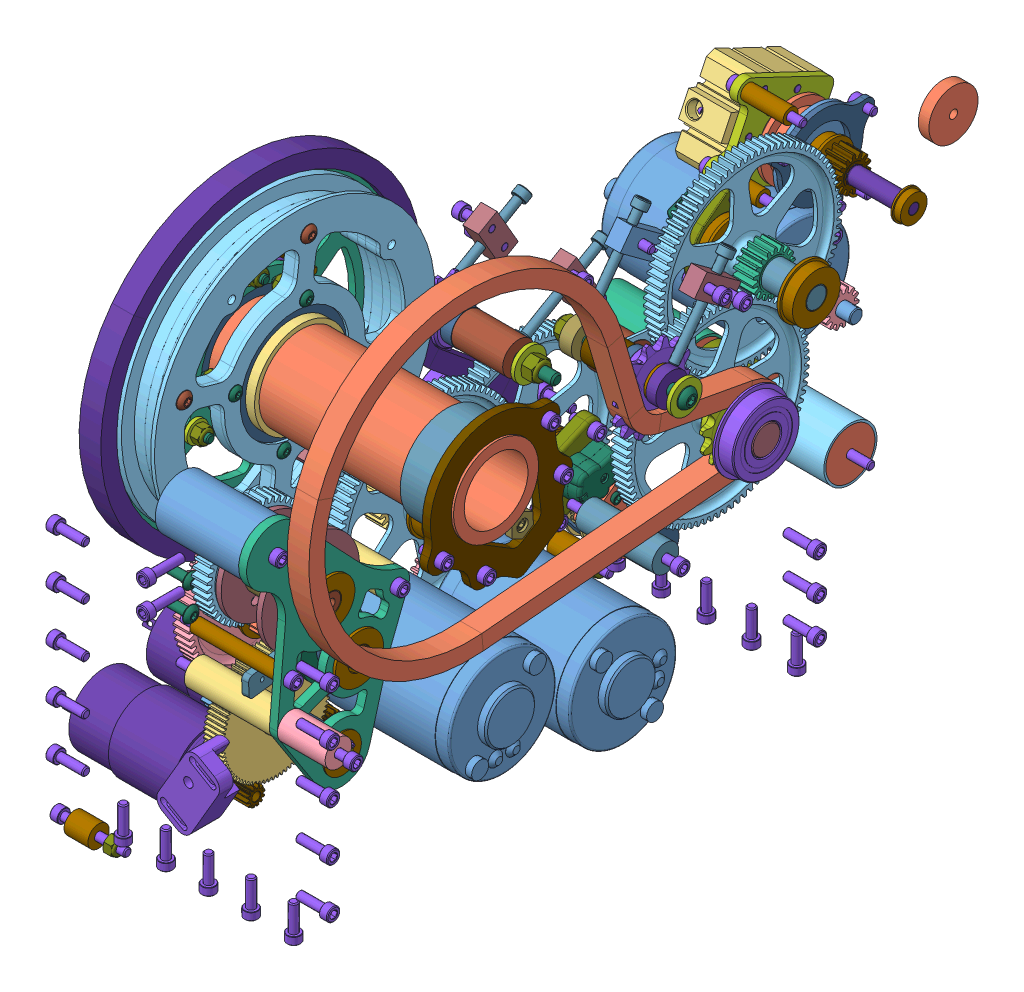
SolidWorks assembly 971-18-A-2900_Arm Gearbox, configuration Default. Lengths in mm. (continued)
Components (placement in the parent): (continued)
- SHCS-20: SHCS [0.4375, #10-32] at (157.9562 -11.0066 -39.4138) x (-1 0 0) z (0 -0.010983 -0.99994) size (16.17 7.92 7.92)
- SHCS-21: SHCS [0.4375, #10-32] at (157.9562 -40.3824 6.6222) x (-1 0 0) z (0 -0.010983 -0.99994) size (16.17 7.92 7.92)
- SHCS-22: SHCS [0.4375, #10-32] at (157.9562 -20.3652 31.9152) x (-1 0 0) z (0 -0.010983 -0.99994) size (16.17 7.92 7.92)
- SHCS-23: SHCS [0.4375, #10-32] at (0.7937 -20.3652 31.9152) x (1 0 0) z (0 -0.408057 0.912956) size (16.17 7.92 7.92)
- SHCS-24: SHCS [0.4375, #10-32] at (0.7937 -11.0066 -39.4138) x (1 0 0) z (0 -0.408057 0.912956) size (16.17 7.92 7.92)
- SHCS-25: SHCS [0.4375, #10-32] at (0.7937 -40.3824 6.6222) x (1 0 0) z (0 -0.408057 0.912956) size (16.17 7.92 7.92)
- SHCS-26: SHCS [0.4375, #10-32] at (0.7937 20.3652 -31.9152) x (1 0 0) z (0 -0.408057 0.912956) size (16.17 7.92 7.92)
- SHCS-27: SHCS [0.625, #10-32] at (150.8125 -172.339 95.6183) x (-1 0 0) z (0 -0.459114 -0.888377) size (20.93 7.92 7.92)
- SHCS-28: SHCS [0.625, #10-32] at (7.9375 -172.339 95.6183) x (1 0 0) z (0 0.669781 0.742559) size (20.93 7.92 7.92)
- SHCS-29: SHCS [0.625, #10-32] at (150.8125 -142.6527 95.6183) x (-1 0 0) z (0 -0.459114 -0.888377) size (20.93 7.92 7.92)
- SHCS-30: SHCS [0.625, #10-32] at (150.8125 -112.9665 95.6183) x (-1 0 0) z (0 -0.459114 -0.888377) size (20.93 7.92 7.92)
- SHCS-31: SHCS [0.625, #10-32] at (150.8125 -83.2802 95.6183) x (-1 0 0) z (0 -0.459114 -0.888377) size (20.93 7.92 7.92)
- SHCS-32: SHCS [0.625, #10-32] at (150.8125 -53.594 95.6183) x (-1 0 0) z (0 -0.459114 -0.888377) size (20.93 7.92 7.92)
- SHCS-33: SHCS [0.625, #10-32] at (7.9375 -142.6527 95.6183) x (1 0 0) z (0 0.669781 0.742559) size (20.93 7.92 7.92)
- SHCS-34: SHCS [0.625, #10-32] at (7.9375 -112.9665 95.6183) x (1 0 0) z (0 0.669781 0.742559) size (20.93 7.92 7.92)
- SHCS-35: SHCS [0.625, #10-32] at (7.9375 -83.2802 95.6183) x (1 0 0) z (0 0.669781 0.742559) size (20.93 7.92 7.92)
- SHCS-36: SHCS [0.625, #10-32] at (7.9375 -53.594 95.6183) x (1 0 0) z (0 0.669781 0.742559) size (20.93 7.92 7.92)
- SHCS-37: SHCS [0.625, #10-32] at (150.8125 -175.26 -195.2625) x (-1 0 0) z (0 -0.430535 -0.902574) size (20.93 7.92 7.92)
- SHCS-38: SHCS [0.625, #10-32] at (7.9375 -175.26 -195.2625) x (1 0 0) z (0 0.669781 0.742559) size (20.93 7.92 7.92)
- SHCS-39: SHCS [0.625, #10-32] at (7.9375 -152.7175 -195.2625) x (1 0 0) z (0 0.669781 0.742559) size (20.93 7.92 7.92)
- SHCS-40: SHCS [0.625, #10-32] at (7.9375 -130.175 -195.2625) x (1 0 0) z (0 0.669781 0.742559) size (20.93 7.92 7.92)
- SHCS-41: SHCS [0.625, #10-32] at (150.8125 -152.7175 -195.2625) x (-1 0 0) z (0 -0.430535 -0.902574) size (20.93 7.92 7.92)
- SHCS-42: SHCS [0.625, #10-32] at (150.8125 -130.175 -195.2625) x (-1 0 0) z (0 -0.430535 -0.902574) size (20.93 7.92 7.92)
- SHCS-46: SHCS [0.625, #10-32] at (139.6577 -185.0517 95.6183) x (0 1 0) z (-0.080041 0 -0.996792) size (20.93 7.92 7.92)
- SHCS-47: SHCS [0.625, #10-32] at (114.2153 -185.0517 95.6183) x (0 1 0) z (-0.080041 0 -0.996792) size (20.93 7.92 7.92)
- SHCS-48: SHCS [0.625, #10-32] at (88.773 -185.0517 95.6183) x (0 1 0) z (-0.266457 0 -0.963847) size (20.93 7.92 7.92)
- SHCS-49: SHCS [0.625, #10-32] at (63.3307 -185.0517 95.6183) x (0 1 0) z (-0.467971 0 -0.883744) size (20.93 7.92 7.92)
- SHCS-50: SHCS [0.625, #10-32] at (37.8883 -185.0517 95.6183) x (0 1 0) z (-0.662108 0 -0.749409) size (20.93 7.92 7.92)
- SHCS-52: SHCS [0.625, #10-32] at (122.2375 -186.4995 -195.2625) x (0 1 0) z (-0.080041 0 -0.996792) size (20.93 7.92 7.92)
- SHCS-53: SHCS [0.625, #10-32] at (95.25 -186.4995 -195.2625) x (0 1 0) z (-0.080041 0 -0.996792) size (20.93 7.92 7.92)
- SHCS-54: SHCS [0.625, #10-32] at (149.225 -186.4995 -195.2625) x (0 1 0) z (-0.266457 0 -0.963847) size (20.93 7.92 7.92)
- SHCS-55: SHCS [0.625, #10-32] at (68.2625 -186.4995 -195.2625) x (0 1 0) z (-0.467971 0 -0.883744) size (20.93 7.92 7.92)
- SHCS-56: SHCS [0.625, #10-32] at (41.275 -186.4995 -195.2625) x (0 1 0) z (-0.662108 0 -0.749409) size (20.93 7.92 7.92)
- SHCS-61: SHCS [1.5, #10-32] at (19.05 -204.4065 -195.2752) x (1 0 0) z (0 0.916141 -0.400857) size (43.15 7.92 7.92)
- No 10 Aluminum Spacer-8: No 10 Aluminum Spacer [0.5" OD, 0.5625" Length] at (13.4938 -204.4065 -195.2752) x (0 0.977573 -0.210597) z (1 0 0) size (12.7 12.7 14.29)
- SHCS-65: SHCS [0.625, #10-32] at (7.9375 -12.5246 -146.6125) x (1 0 0) z (0 -0.814974 -0.579498) size (20.93 7.92 7.92)
- SHCS-67: SHCS [0.625, #10-32] at (7.9375 -25.7229 -154.2325) x (1 0 0) z (0 -0.96514 -0.261734) size (20.93 7.92 7.92)
- SHCS-69: SHCS [0.625, #10-32] at (100.3427 21.0025 -150.0962) x (1 0 0) z (0 -0.52095 -0.853587) size (20.93 7.92 7.92)
- SHCS-71: SHCS [0.625, #10-32] at (100.3427 13.4742 -160.3243) x (1 0 0) z (0 -0.512621 -0.858615) size (20.93 7.92 7.92)
- 971-18-P-0243_Arm Gearbox Potentiometer Mount-2: 971-18-P-0243_Arm Gearbox Potentiometer Mount [Default] at (100.4062 -85.7984 -149.5368) x (0 0.994332 -0.106322) z (-1 0 0) size (42.8 25.4 21.27)
- VexPro_Hex Spacers-1: VexPro_Hex Spacers [1_2 Hex, 0.5] at (114.7839 -58.42 -165.2367) x (0 0 -1) z (1 0 0) size (19.51 19.51 12.7)
- SHCS-76: SHCS [0.625, #10-32] at (150.8125 29.2837 -138.8453) x (-1 0 0) z (0 -0.37606 -0.926595) size (20.93 7.92 7.92)
- SHCS-78: SHCS [0.625, #10-32] at (150.8125 20.2497 -151.119) x (-1 0 0) z (0 -0.490985 -0.871168) size (20.93 7.92 7.92)
- SHCS-80: SHCS [0.625, #10-32] at (60.325 -12.5246 -146.6125) x (-1 0 0) z (0 -0.909347 -0.416039) size (20.93 7.92 7.92)
- SHCS-82: SHCS [0.625, #10-32] at (60.325 -25.7229 -154.2325) x (-1 0 0) z (0 -0.967776 -0.251812) size (20.93 7.92 7.92)
- VexPro_Hex Spacers-2: VexPro_Hex Spacers [1_2 Hex, 0.0625] at (61.1187 -103.4997 -135.089) x (0 0.01328 -0.999912) z (1 0 0) size (19.51 19.51 1.59)
- 971-18-P-0249_Distal Shaft Spacer-1: 971-18-P-0249_Distal Shaft Spacer [Default] at (26.5543 -103.4997 -135.089) size (9.91 19.5 19.5)
- Nylon-Insert Locknut-3: Nylon-Insert Locknut [#8-32  Nylon-Insert Locknut] at (27.686 -204.4065 -195.2752) x (0 0.839079 -0.544009) z (0 -0.544009 -0.839079) size (8.73 5.95 10.08)
- No 10 Aluminum Spacer-9: No 10 Aluminum Spacer [0.5" OD, 0.5625" Length] at (13.4938 -204.4065 93.1418) x (0 0.977573 -0.210597) z (1 0 0) size (12.7 12.7 14.29)
- No 10 Aluminum Spacer-10: No 10 Aluminum Spacer [0.5" OD, 0.5625" Length] at (13.4938 -204.4065 -145.3959) x (0 0.977573 -0.210597) z (1 0 0) size (12.7 12.7 14.29)
- No 10 Aluminum Spacer-11: No 10 Aluminum Spacer [0.5" OD, 0.5625" Length] at (13.4938 -204.4065 -95.5167) x (0 0.977573 -0.210597) z (1 0 0) size (12.7 12.7 14.29)
- No 10 Aluminum Spacer-12: No 10 Aluminum Spacer [0.5" OD, 0.5625" Length] at (13.4938 -204.4065 -6.6167) x (0 0.977573 -0.210597) z (1 0 0) size (12.7 12.7 14.29)
- SHCS-84: SHCS [1.5, #10-32] at (19.05 -204.4065 93.1418) x (1 0 0) z (0 0.916141 -0.400857) size (43.15 7.92 7.92)
- SHCS-85: SHCS [1.5, #10-32] at (19.05 -204.4065 -145.3959) x (1 0 0) z (0 0.916141 -0.400857) size (43.15 7.92 7.92)
- SHCS-86: SHCS [1.5, #10-32] at (19.05 -204.4065 -95.5167) x (1 0 0) z (0 0.916141 -0.400857) size (43.15 7.92 7.92)
- SHCS-87: SHCS [1.5, #10-32] at (19.05 -204.4065 -6.6167) x (1 0 0) z (0 0.916141 -0.400857) size (43.15 7.92 7.92)
- Nylon-Insert Locknut-4: Nylon-Insert Locknut [#8-32  Nylon-Insert Locknut] at (27.686 -204.4065 93.1418) x (0 0.839079 -0.544009) z (0 -0.544009 -0.839079) size (8.73 5.95 10.08)
- Nylon-Insert Locknut-5: Nylon-Insert Locknut [#8-32  Nylon-Insert Locknut] at (27.686 -204.4065 -145.3959) x (0 0.839079 -0.544009) z (0 -0.544009 -0.839079) size (8.73 5.95 10.08)
- Nylon-Insert Locknut-6: Nylon-Insert Locknut [#8-32  Nylon-Insert Locknut] at (27.686 -204.4065 -95.5167) x (0 0.839079 -0.544009) z (0 -0.544009 -0.839079) size (8.73 5.95 10.08)
- Nylon-Insert Locknut-7: Nylon-Insert Locknut [#8-32  Nylon-Insert Locknut] at (27.686 -204.4065 -6.6167) x (0 0.839079 -0.544009) z (0 -0.544009 -0.839079) size (8.73 5.95 10.08)
- BHCS-3: BHCS [0.5625, #10-32] at (70.8279 -51.689 86.0933) x (0 -0.746359 0.665543) z (1 0 0) size (9.17 9.17 17.04)
- BHCS-4: BHCS [0.5625, #10-32] at (70.8279 -69.1515 86.0933) x (0 -0.746359 0.665543) z (1 0 0) size (9.17 9.17 17.04)
- SHCS-88: SHCS [0.75, #10-32] at (58.7375 -46.9265 90.8558) x (0 0 -1) z (0.742559 0.669781 0) size (24.1 7.92 7.92)
- SHCS-89: SHCS [0.75, #10-32] at (58.7375 -64.389 90.8558) x (0 0 -1) z (0.742559 0.669781 0) size (24.1 7.92 7.92)
- BHCS-6: BHCS [0.5, #10-32] at (77.2604 -134.8658 -152.2116) x (0 0.490356 0.871522) z (1 0 0) size (9.17 9.17 15.45)
- BHCS-7: BHCS [0.5, #10-32] at (77.2604 -128.7793 -160.3468) x (0 0.345971 0.938245) z (1 0 0) size (9.17 9.17 15.45)
- 91525A416_1-4 Oversized Washer-1: 91525A416_1-4 Oversized Washer [91525A416] at (-2.286 -39.637 -114.8895) size (2.29 19.05 19.05)
- 91525A416_1-4 Oversized Washer-2: 91525A416_1-4 Oversized Washer [91525A416] at (68.2625 -39.637 -114.8895) size (2.29 19.05 19.05)
- 91525A416_1-4 Oversized Washer-3: 91525A416_1-4 Oversized Washer [91525A416] at (158.75 -12.6592 -117.4327) size (2.29 19.05 19.05)
- 971-18-P-0057_Arm Gearbox Plates-2: 971-18-P-0057_Arm Gearbox Plates [Sponsor Pannel Outside] at (4.826 0 0) size (0.81 228.95 407.67) (hidden)
- 971-18-P-0057_Arm Gearbox Plates-3: 971-18-P-0057_Arm Gearbox Plates [Sponsor Pannel Inside] at (-4.826 0 0) size (0.81 222.6 407.67) (hidden)
- 971-18-P-0352_Arm Gearbox-Bumper Spacer-1: 971-18-P-0352_Arm Gearbox-Bumper Spacer [Default] at (90.8758 -115.2621 108.5723) x (0 0 -1) z (-0.864092 0.503334 0) size (17.72 44.45 22.86)
Mates (geometry in assembly coordinates):
- Concentric17: concentric anti-aligned: cylinder of MiniCIM-1 through (184.5808 -45.1539 -242.57) axis (-1 0 0) radius 32.131; cylinder of 971-18-P-0057_Arm Gearbox Plates-1 through (101.9302 -45.1539 -242.57) axis (1 0 0) radius 9.5631
- Concentric10: concentric anti-aligned: cylinder of MiniCIM-2 through (68.2625 -128.7803 -15.3525) axis (1 0 0) radius 4; cylinder of 14T-CIM_217-3414-1 through (44.9112 -128.7803 -15.3525) axis (-1 0 0) radius 4
- Concentric11: concentric anti-aligned: cylinder of 971-18-P-0057_Arm Gearbox Plates-1 through (68.2625 -91.1077 -64.9795) axis (-1 0 0) radius 14.2684; cylinder of 971-18-P-0186_84T Gear With Access Hole-2 through (49.2633 -91.1077 -64.9795) axis (1 0 0) radius 8.89
- Concentric21: concentric anti-aligned: cylinder of 971-18-P-0057_Arm Gearbox Plates-1 through (158.75 -58.42 -165.2367) axis (-1 0 0) radius 19.981; cylinder of 971-18-P-0186_84T Gear With Access Hole-4 through (121.1339 -58.42 -165.2367) axis (1 0 0) radius 8.89
- Concentric22: concentric anti-aligned: cylinder of 971-18-P-0057_Arm Gearbox Plates-1 through (158.75 -2.1568 -197.4778) axis (-1 0 0) radius 14.2684; cylinder of 18T-1_2-Hex-Steel_217-5460-2 through (121.1339 -2.1568 -197.4778) axis (1 0 0) radius 8.89
- Concentric12: concentric anti-aligned: cylinder of 28T-1_2-Hex-Steel_217-5468-1 through (49.2633 -91.1077 -64.9795) axis (-1 0 0) radius 8.89; cylinder of 971-18-P-0186_84T Gear With Access Hole-2 through (49.2633 -91.1077 -64.9795) axis (1 0 0) radius 8.89
- Concentric23: concentric aligned: cylinder of 971-18-P-0186_84T Gear With Access Hole-3 through (108.4848 -2.1568 -197.4778) axis (1 0 0) radius 8.89; cylinder of 18T-1_2-Hex-Steel_217-5460-2 through (121.1339 -2.1568 -197.4778) axis (1 0 0) radius 8.89
- Coincident29: coincident aligned: plane of 971-18-P-0186_84T Gear With Access Hole-4 through (121.1339 -58.42 -165.2367) normal (-1 0 0); plane of 18T-1_2-Hex-Steel_217-5460-2 through (121.1339 -2.1568 -197.4778) normal (-1 0 0)
- Coincident31: coordinate: point of 971-18-P-0057_Arm Gearbox Plates-1
- Concentric24: concentric anti-aligned: cylinder of 971-18-P-0057_Arm Gearbox Plates-1 through (6.35 0 0) axis (-1 0 0) radius 25; cylinder of 971-18-P-0063_Proximal Joint Chain-1 through (142.3112 0 0) axis (1 0 0) radius 95.7195
- Concentric30: concentric anti-aligned: cylinder of MiniCIM-3 through (68.2625 -149.225 -87.4394) axis (1 0 0) radius 4; cylinder of 14T-CIM_217-3414-2 through (44.9112 -149.225 -87.4394) axis (-1 0 0) radius 4
- Concentric31: concentric aligned: cylinder of MiniCIM-1 through (101.9302 -45.1539 -242.57) axis (-1 0 0) radius 4; cylinder of 14T-CIM_217-3414-3 through (119.605 -45.1539 -242.57) axis (-1 0 0) radius 4
- Concentric33: concentric aligned: cylinder of 971-18-P-0057_Arm Gearbox Plates-1 through (6.35 -91.1077 -64.9795) axis (-1 0 0) radius 14.2684; cylinder of Bearings-2 through (-1.9181 -91.1077 -64.9795) axis (-1 0 0) radius 14.2875
- Concentric35: concentric anti-aligned: cylinder of 971-18-P-0057_Arm Gearbox Plates-1 through (158.75 -2.1568 -197.4778) axis (-1 0 0) radius 14.2684; cylinder of Bearings-4 through (160.6681 -2.1568 -197.4778) axis (1 0 0) radius 14.2875
- Coincident42: coincident anti-aligned: plane of 971-18-P-0057_Arm Gearbox Plates-1 through (106.6927 0 0) normal (1 0 0); plane of Bearings-5 through (106.6927 1.0288 -211.4056) normal (-1 0 0)
- Concentric36: concentric anti-aligned: cylinder of 971-18-P-0057_Arm Gearbox Plates-1 through (101.9302 -2.1568 -197.4778) axis (1 0 0) radius 14.2684; cylinder of Bearings-5 through (93.2501 -2.1568 -197.4778) axis (-1 0 0) radius 15.5575
- Concentric37: concentric anti-aligned: cylinder of 971-18-P-0057_Arm Gearbox Plates-1 through (68.2625 -91.1077 -64.9795) axis (-1 0 0) radius 14.2684; cylinder of Bearings-6 through (71.7681 -91.1077 -64.9795) axis (1 0 0) radius 14.2875
- Coincident43: coincident anti-aligned: plane of 971-18-P-0057_Arm Gearbox Plates-1 through (63.5 0 0) normal (-1 0 0); plane of Bearings-6 through (63.5 -102.311 -56.1128) normal (1 0 0)
- Concentric2: concentric anti-aligned: cylinder of 12T_Hex_217-2662-5 through (133.7831 -58.42 -165.2367) axis (1 0 0) radius 12.7; cylinder of 6661K350_17mm ID 40mm OD BALL BEARING-3 through (149.22 -58.42 -165.2367) axis (-1 0 0) radius 20
- Coincident3: coincident anti-aligned: plane of 971-18-P-0057_Arm Gearbox Plates-1 through (152.4 0 0) normal (-1 0 0); plane of 6661K350_17mm ID 40mm OD BALL BEARING-3 through (152.4 -66.9352 -144.6265) normal (1 0 0)
- Concentric44: concentric aligned: cylinder of 971-18-P-0057_Arm Gearbox Plates-1 through (158.75 -58.42 -165.2367) axis (-1 0 0) radius 19.981; cylinder of 6661K350_17mm ID 40mm OD BALL BEARING-3 through (149.22 -58.42 -165.2367) axis (-1 0 0) radius 20
- Concentric46: concentric anti-aligned: cylinder of 971-18-P-0057_Arm Gearbox Plates-1 through (6.35 -103.4997 -135.089) axis (-1 0 0) radius 19.981; cylinder of 6661K350_17mm ID 40mm OD BALL BEARING-2 through (9.53 -103.4997 -135.089) axis (1 0 0) radius 20
- Coincident57: coincident anti-aligned: plane of 971-18-P-0057_Arm Gearbox Plates-1 through (6.35 0 0) normal (1 0 0); plane of 6661K350_17mm ID 40mm OD BALL BEARING-2 through (6.35 -125.7997 -135.089) normal (-1 0 0)
- Concentric47: concentric anti-aligned: cylinder of 12T_Hex_217-2662-2 through (26.5543 -103.4997 -135.089) axis (-1 0 0) radius 12.7; cylinder of 6661K350_17mm ID 40mm OD BALL BEARING-2 through (9.53 -103.4997 -135.089) axis (1 0 0) radius 20
- Coincident59: coincident anti-aligned: plane of 971-18-P-0057_Arm Gearbox Plates-1 through (68.2625 0 0) normal (1 0 0); plane of MiniCIM-2 through (68.2625 -135.2517 -22.3416) normal (-1 0 0)
- Coincident60: coincident anti-aligned: plane of 971-18-P-0057_Arm Gearbox Plates-1 through (68.2625 0 0) normal (1 0 0); plane of MiniCIM-3 through (68.2625 -143.5324 -95.0761) normal (-1 0 0)
- Concentric49: concentric anti-aligned: cylinder of 971-18-P-0057_Arm Gearbox Plates-1 through (68.2625 -149.225 -87.4394) axis (-1 0 0) radius 9.5631; cylinder of MiniCIM-3 through (-14.3881 -149.225 -87.4394) axis (1 0 0) radius 32.131
- Coincident61: coincident aligned: plane of 14T-CIM_217-3414-1 through (35.3862 -128.7803 -15.3525) normal (-1 0 0); plane of 14T-CIM_217-3414-2 through (35.3862 -149.225 -87.4394) normal (-1 0 0)
- Width7: width anti-aligned: plane of 12T_Hex_217-2662-5 through (140.1649 -58.42 -165.2367) normal (-1 0 0); plane of 12T_Hex_217-2662-5 through (144.4575 -42.574 -164.3842) normal (1 0 0); plane of 971-18-P-0063_Proximal Joint Chain-1 through (148.7882 -81.2845 -167.2612) normal (1 0 0); plane of 971-18-P-0063_Proximal Joint Chain-1 through (135.8342 -81.2845 -167.2612) normal (-1 0 0)
- Coincident62: coincident aligned: plane of 28T-1_2-Hex-Steel_217-5468-1 through (36.6633 -91.1077 -64.9795) normal (-1 0 0); plane of 971-18-P-0186_84T Gear With Access Hole-1 through (36.6633 -103.4997 -135.089) normal (-1 0 0)
- Coincident63: coincident anti-aligned: plane of 28T-1_2-Hex-Steel_217-5468-1 through (49.2633 -91.1077 -64.9795) normal (1 0 0); plane of 971-18-P-0186_84T Gear With Access Hole-2 through (49.2633 -91.1077 -64.9795) normal (-1 0 0)
- Coincident64: coincident anti-aligned: plane of 971-18-P-0186_84T Gear With Access Hole-2 through (61.9125 -91.1077 -64.9795) normal (1 0 0); plane of Bearings-6 through (61.9125 -102.311 -56.1128) normal (-1 0 0)
- Coincident66: coincident anti-aligned: plane of 971-18-P-0057_Arm Gearbox Plates-1 through (101.9302 0 0) normal (-1 0 0); plane of MiniCIM-1 through (101.9302 -37.301 -247.9604) normal (1 0 0)
- Concentric55: concentric anti-aligned: cylinder of 971-18-P-0063_Proximal Joint Chain-1 through (142.3112 -58.42 -165.2367) axis (1 0 0) radius 22.9539; cylinder of 6661K350_17mm ID 40mm OD BALL BEARING-3 through (149.22 -58.42 -165.2367) axis (-1 0 0) radius 8.5
- Concentric62: concentric anti-aligned: cylinder of 971-18-P-0057_Arm Gearbox Plates-1 through (101.9302 -58.42 -165.2367) axis (1 0 0) radius 14.2684; cylinder of 3547S-1AA-102A-ND 3 Turn Potentiometer Bourns-2 through (103.1711 -58.42 -165.2367) axis (-1 0 0) radius 3.175
- Coincident72: coincident anti-aligned: plane of 971-18-P-0057_Arm Gearbox Plates-1 through (152.4 0 0) normal (-1 0 0); plane of Bearings-4 through (152.4 -15.7305 -201.9373) normal (1 0 0)
- Concentric64: concentric anti-aligned: cylinder of 971-18-P-0057_Arm Gearbox Plates-1 through (68.2625 -103.4997 -135.089) axis (-1 0 0) radius 14.2684; cylinder of Bearings-1 through (71.7681 -103.4997 -135.089) axis (1 0 0) radius 14.2875
- Coincident73: coincident anti-aligned: plane of 971-18-P-0057_Arm Gearbox Plates-1 through (63.5 0 0) normal (-1 0 0); plane of Bearings-1 through (63.5 -89.5132 -138.0061) normal (1 0 0)
- Concentric65: concentric anti-aligned: cylinder of 971-18-P-0057_Arm Gearbox Plates-1 through (101.9302 -58.42 -165.2367) axis (1 0 0) radius 14.2684; cylinder of Bearings-9 through (98.4246 -58.42 -165.2367) axis (-1 0 0) radius 14.2875
- Coincident74: coincident anti-aligned: plane of 971-18-P-0057_Arm Gearbox Plates-1 through (106.6927 0 0) normal (1 0 0); plane of Bearings-9 through (106.6927 -59.4815 -150.9887) normal (-1 0 0)
- Concentric67: concentric anti-aligned: cylinder of Bearings-1 through (71.7681 -103.4997 -135.089) axis (1 0 0) radius 6.35; cylinder of SRK Mag Encoder Magnet-1 through (75.7047 -103.4997 -135.089) axis (-1 0 0) radius 3.175
- Concentric68: concentric anti-aligned: cylinder of Bearings-5 through (98.4246 -2.1568 -197.4778) axis (-1 0 0) radius 6.35; cylinder of SRK Mag Encoder Magnet-2 through (94.5515 -2.1568 -197.4778) axis (1 0 0) radius 3.175
- Concentric70: concentric aligned: cylinder of 6661K350_17mm ID 40mm OD BALL BEARING-3 through (149.22 -58.42 -165.2367) axis (-1 0 0) radius 8.5; cylinder of 971-18-P-0104_Arm Gearbox Proximal Arm Output Shaft-1 through (161.22 -58.42 -165.2367) axis (-1 0 0) radius 8.5
- Coincident80: coincident anti-aligned: plane of 6661K350_17mm ID 40mm OD BALL BEARING-3 through (149.22 -63.3914 -153.204) normal (-1 0 0); plane of 971-18-P-0104_Arm Gearbox Proximal Arm Output Shaft-1 through (149.22 -63.3153 -158.2879) normal (1 0 0)
- Coincident81: coincident anti-aligned: plane of 12T_Hex_217-2662-5 through (144.4575 -42.574 -164.3842) normal (1 0 0); plane of 971-18-P-0104_Arm Gearbox Proximal Arm Output Shaft-1 through (144.4575 -63.9057 -157.45) normal (-1 0 0)
- Coincident82: coincident anti-aligned: plane of 971-18-P-0186_84T Gear With Access Hole-4 through (133.7831 -58.42 -165.2367) normal (1 0 0); plane of 12T_Hex_217-2662-5 through (133.7831 -58.42 -165.2367) normal (-1 0 0)
- Concentric71: concentric anti-aligned: cylinder of Bearings-4 through (160.6681 -2.1568 -197.4778) axis (1 0 0) radius 6.35; cylinder of 971-18-P-0105_Arm Gearbox Proximal Arm First Stage Shaft -1 through (133.7437 -2.1568 -197.4778) axis (-1 0 0) radius 6.35
- Coincident83: coincident anti-aligned: plane of Bearings-4 through (150.8125 -15.7305 -201.9373) normal (-1 0 0); plane of 971-18-P-0105_Arm Gearbox Proximal Arm First Stage Shaft -1 through (150.8125 4.1932 -197.4778) normal (1 0 0)
- Concentric72: concentric anti-aligned: cylinder of 6661K350_17mm ID 40mm OD BALL BEARING-2 through (9.53 -103.4997 -135.089) axis (1 0 0) radius 8.5; cylinder of 971-18-P-0107_Arm Gearbox Distal Arm Output Shaft-1 through (69.8627 -103.4997 -135.089) axis (-1 0 0) radius 8.5
- Coincident84: coincident anti-aligned: plane of 6661K350_17mm ID 40mm OD BALL BEARING-2 through (9.53 -116.519 -135.089) normal (1 0 0); plane of 971-18-P-0107_Arm Gearbox Distal Arm Output Shaft-1 through (9.53 -94.7353 -131.3594) normal (-1 0 0)
- Coincident85: coincident anti-aligned: plane of 12T_Hex_217-2662-2 through (15.88 -90.4408 -144.1049) normal (-1 0 0); plane of 971-18-P-0107_Arm Gearbox Distal Arm Output Shaft-1 through (15.88 -96.4882 -132.1053) normal (1 0 0)
- Concentric73: concentric aligned: cylinder of Bearings-2 through (-1.9181 -91.1077 -64.9795) axis (-1 0 0) radius 6.35; cylinder of 971-18-P-0106_Arm Gearbox Distal Arm First Stage Shaft-1 through (69.8627 -91.1077 -64.9795) axis (-1 0 0) radius 6.35
- Coincident86: coincident anti-aligned: plane of 971-18-P-0057_Arm Gearbox Plates-1 through (6.35 0 0) normal (1 0 0); plane of Bearings-2 through (6.35 -103.9479 -58.7135) normal (-1 0 0)
- Coincident87: coincident anti-aligned: plane of Bearings-2 through (7.9375 -103.9479 -58.7135) normal (1 0 0); plane of 971-18-P-0106_Arm Gearbox Distal Arm First Stage Shaft-1 through (7.9375 -83.1702 -64.9795) normal (-1 0 0)
- Concentric74: concentric anti-aligned: cylinder of 12T_Hex_217-2662-2 through (26.5543 -103.4997 -135.089) axis (-1 0 0) radius 12.7; cylinder of 971-18-P-0070_Distal Joint Chain-1 through (18.0263 -103.4997 -135.089) axis (1 0 0) radius 13.4289
- Concentric75: concentric anti-aligned: cylinder of 971-18-P-0057_Arm Gearbox Plates-1 through (6.35 0 0) axis (-1 0 0) radius 25; cylinder of 971-18-P-0070_Distal Joint Chain-1 through (18.0263 0 0) axis (1 0 0) radius 95.7195
- Width8: width anti-aligned: plane of 12T_Hex_217-2662-2 through (15.88 -90.4408 -144.1049) normal (-1 0 0); plane of 12T_Hex_217-2662-2 through (20.1726 -103.4997 -135.089) normal (1 0 0); plane of 971-18-P-0070_Distal Joint Chain-1 through (24.5033 -85.8001 -149.7042) normal (1 0 0); plane of 971-18-P-0070_Distal Joint Chain-1 through (11.5493 -85.8001 -149.7042) normal (-1 0 0)
- Concentric76: concentric anti-aligned: cylinder of 971-18-P-0057_Arm Gearbox Plates-1 through (6.35 0 0) axis (-1 0 0) radius 25; cylinder of 971-18-P-0101_Tensioner Strap-1 through (-4.7625 0 0) axis (1 0 0) radius 25
- Coincident88: coincident anti-aligned: plane of 971-18-P-0057_Arm Gearbox Plates-1 through (0 0 0) normal (-1 0 0); plane of 971-18-P-0101_Tensioner Strap-1 through (0 0 0) normal (1 0 0)
- Concentric77: concentric anti-aligned: cylinder of 971-18-P-0057_Arm Gearbox Plates-1 through (158.75 0 0) axis (-1 0 0) radius 25; cylinder of 971-18-P-0101_Tensioner Strap-2 through (158.75 0 0) axis (1 0 0) radius 25
- Coincident89: coincident anti-aligned: plane of 971-18-P-0057_Arm Gearbox Plates-1 through (158.75 0 0) normal (1 0 0); plane of 971-18-P-0101_Tensioner Strap-2 through (158.75 0 0) normal (-1 0 0)
- Coincident90: coincident aligned: plane of 971-18-P-0101_Tensioner Strap-1 through (-4.7625 -29.9915 -25.9171) normal (0 0.842996 0.537919); plane of 971-18-P-0101_Tensioner Strap-2 through (158.75 -29.9915 -25.9171) normal (0 0.842996 0.537919)
- Concentric79: concentric anti-aligned: cylinder of 3549S-1BA-102B-ND 10 turn potentiometer-1 through (54.078 -149.8585 -169.7731) axis (1 0 0) radius 3.175; cylinder of potentiometer belt-1 through (58.0437 -149.8585 -169.7731) axis (-1 0 0) radius 12.2725
- Concentric81: concentric aligned: cylinder of 3549S-1BA-102B-ND 10 turn potentiometer-1 through (74.695 -149.8585 -169.7731) axis (1 0 0) radius 11.2395; cylinder of 971-18-P-0112_Arm Gearbox Distal Potentiometer Mount-1 through (68.345 -149.8585 -169.7731) axis (1 0 0) radius 5.1753
- Concentric83: concentric aligned: cylinder of 3549S-1BA-102B-ND 10 turn potentiometer-1 through (54.078 -149.8585 -169.7731) axis (1 0 0) radius 3.175; cylinder of A-6z16-036df2508_36t plastic pulley-1 through (60.425 -149.8585 -169.7731) axis (1 0 0) radius 8.7312
- Width9: width anti-aligned: plane of A-6z16-036df2508_36t plastic pulley-1 through (49.3125 -149.8585 -169.7731) normal (-1 0 0); plane of A-6z16-036df2508_36t plastic pulley-1 through (60.425 -149.8585 -169.7731) normal (1 0 0); plane of potentiometer belt-1 through (58.0437 -103.4997 -135.089) normal (1 0 0); plane of potentiometer belt-1 through (51.6937 -103.4997 -135.089) normal (-1 0 0)
- Concentric84: concentric aligned: cylinder of potentiometer belt-1 through (58.0437 -103.4997 -135.089) axis (-1 0 0) radius 13.5661; cylinder of 971-18-P-0254_40T plastic pulley hex-1 through (60.9806 -103.4997 -135.089) axis (-1 0 0) radius 12.7
- Width10: width aligned: plane of 971-18-P-0254_40T plastic pulley hex-1 through (58.8375 -103.4997 -135.089) normal (-1 0 0); plane of 971-18-P-0254_40T plastic pulley hex-1 through (50.9 -103.4997 -135.089) normal (1 0 0); plane of potentiometer belt-1 through (51.6937 -103.4997 -135.089) normal (-1 0 0); plane of potentiometer belt-1 through (58.0437 -103.4997 -135.089) normal (1 0 0)
- Concentric85: concentric anti-aligned: cylinder of 971-18-P-0063_Proximal Joint Chain-1 through (142.3112 -12.6592 -117.4327) axis (-1 0 0) radius 13.4289; cylinder of 971-18-A-4500_Arm Tensioner Idler-1/971-18-P-0119_Arm Tensioner Idler-1 through (133.7831 -12.6592 -117.4327) axis (1 0 0) radius 12.7
- Coincident97: coincident aligned: plane of 12T_Hex_217-2662-5 through (144.4575 -42.574 -164.3842) normal (1 0 0); plane of 971-18-A-4500_Arm Tensioner Idler-1/971-18-P-0119_Arm Tensioner Idler-1 through (144.4575 1.0126 -125.4891) normal (1 0 0)
- Concentric86: concentric aligned: cylinder of 971-18-P-0070_Distal Joint Chain-1 through (18.0263 -39.637 -114.8895) axis (-1 0 0) radius 13.4289; cylinder of 971-18-A-4500_Arm Tensioner Idler-2/8491A293_0_5 OD PRESS-FIT DRILL BUSHING-1 through (32.9044 -39.637 -114.8895) axis (-1 0 0) radius 3.2639
- Coincident98: coincident aligned: plane of 12T_Hex_217-2662-2 through (15.88 -90.4408 -144.1049) normal (-1 0 0); plane of 971-18-A-4500_Arm Tensioner Idler-2/971-18-P-0119_Arm Tensioner Idler-1 through (15.88 -33.4715 -129.5117) normal (-1 0 0)
- Concentric87: concentric anti-aligned: cylinder of 971-18-A-4500_Arm Tensioner Idler-2/8491A293_0_5 OD PRESS-FIT DRILL BUSHING-1 through (32.9044 -39.637 -114.8895) axis (-1 0 0) radius 3.2639; cylinder of 971-18-P-0122_Distal Tensioner Long Spacer-1 through (69.926 -39.637 -114.8895) axis (1 0 0) radius 9.525
- Coincident99: coincident anti-aligned: plane of 971-18-A-4500_Arm Tensioner Idler-2/8491A293_0_5 OD PRESS-FIT DRILL BUSHING-1 through (32.9044 -39.637 -114.8895) normal (1 0 0); plane of 971-18-P-0122_Distal Tensioner Long Spacer-1 through (32.9044 -30.112 -114.8895) normal (-1 0 0)
- Concentric88: concentric anti-aligned: cylinder of 971-18-A-4500_Arm Tensioner Idler-2/8491A293_0_5 OD PRESS-FIT DRILL BUSHING-1 through (32.9044 -39.637 -114.8895) axis (-1 0 0) radius 3.2639; cylinder of 971-18-P-0123_Distal Tensioner Short Spacer-1 through (31.8387 -39.637 -114.8895) axis (1 0 0) radius 3.2639
- Coincident100: coincident anti-aligned: plane of 971-18-A-4500_Arm Tensioner Idler-2/8491A293_0_5 OD PRESS-FIT DRILL BUSHING-1 through (13.8544 -39.637 -114.8895) normal (-1 0 0); plane of 971-18-P-0123_Distal Tensioner Short Spacer-1 through (13.8544 -30.1475 -115.711) normal (1 0 0)
- Coincident101: coincident anti-aligned: plane of 971-18-P-0057_Arm Gearbox Plates-1 through (6.35 0 0) normal (1 0 0); plane of 971-18-P-0124_Sketchy Chain Tensioner-1 through (6.35 -19.1237 -150.4225) normal (-1 0 0)
- Concentric89: concentric anti-aligned: cylinder of 971-18-P-0057_Arm Gearbox Plates-1 through (0 -12.5246 -146.6125) axis (-1 0 0) radius 2.4892; cylinder of 971-18-P-0124_Sketchy Chain Tensioner-1 through (15.875 -12.5246 -146.6125) axis (1 0 0) radius 2.0193
- Concentric90: concentric anti-aligned: cylinder of 971-18-P-0057_Arm Gearbox Plates-1 through (0 -25.7229 -154.2325) axis (-1 0 0) radius 2.4892; cylinder of 971-18-P-0124_Sketchy Chain Tensioner-1 through (15.875 -25.7229 -154.2325) axis (1 0 0) radius 2.0193
- Concentric91: concentric anti-aligned: cylinder of 971-18-P-0124_Sketchy Chain Tensioner-1 through (11.1125 -15.9487 -155.9218) axis (0 0.5 -0.866025) radius 2.0193; cylinder of 90044A120_2-in Full Thread BLACK-OXIDE ALLOY STEEL SOCKET HEAD CAP SCREW-1 through (11.1125 -9.4758 -167.1332) axis (0 -0.5 0.866025) radius 2.413
- Tangent1: tangent anti-aligned: cylinder of 971-18-P-0123_Distal Tensioner Short Spacer-1 through (31.8387 -39.637 -114.8895) axis (1 0 0) radius 9.525; plane of 90044A120_2-in Full Thread BLACK-OXIDE ALLOY STEEL SOCKET HEAD CAP SCREW-1 through (11.1125 -34.8758 -123.1391) normal (0 -0.5 0.866025)
- Concentric92: concentric anti-aligned: cylinder of 971-18-P-0057_Arm Gearbox Plates-1 through (0 -12.5246 -146.6125) axis (-1 0 0) radius 2.4892; cylinder of 971-18-P-0124_Sketchy Chain Tensioner-2 through (63.5 -12.5246 -146.6125) axis (1 0 0) radius 2.0193
- Concentric93: concentric anti-aligned: cylinder of 971-18-P-0057_Arm Gearbox Plates-1 through (0 -25.7229 -154.2325) axis (-1 0 0) radius 2.4892; cylinder of 971-18-P-0124_Sketchy Chain Tensioner-2 through (63.5 -25.7229 -154.2325) axis (1 0 0) radius 2.0193
- Coincident102: coincident anti-aligned: plane of 971-18-P-0057_Arm Gearbox Plates-1 through (63.5 0 0) normal (-1 0 0); plane of 971-18-P-0124_Sketchy Chain Tensioner-2 through (63.5 -19.1237 -150.4225) normal (1 0 0)
- Concentric94: concentric anti-aligned: cylinder of 971-18-P-0124_Sketchy Chain Tensioner-2 through (58.7375 -15.9487 -155.9218) axis (0 0.5 -0.866025) radius 2.0193; cylinder of 90044A120_2-in Full Thread BLACK-OXIDE ALLOY STEEL SOCKET HEAD CAP SCREW-2 through (58.7375 -9.4758 -167.1332) axis (0 -0.5 0.866025) radius 2.413
- Tangent2: tangent anti-aligned: cylinder of 971-18-P-0122_Distal Tensioner Long Spacer-1 through (69.926 -39.637 -114.8895) axis (1 0 0) radius 9.525; plane of 90044A120_2-in Full Thread BLACK-OXIDE ALLOY STEEL SOCKET HEAD CAP SCREW-2 through (58.7375 -34.8758 -123.1391) normal (0 -0.5 0.866025)
- Concentric99: concentric anti-aligned: cylinder of BHCS-1 through (86.614 -39.637 -114.8895) axis (1 0 0) radius 3.175; cylinder of Nylon-Insert Locknut-1 through (67.3735 -39.637 -114.8895) axis (-1 0 0) radius 3.175
- Concentric100: concentric anti-aligned: cylinder of 971-18-A-4500_Arm Tensioner Idler-1/5905K230_0_5ID STEEL NEEDLE-ROLLER BEARING-1 through (133.7831 -12.6592 -117.4327) axis (-1 0 0) radius 8.7312; cylinder of 971-18-P-0248_Proximal Tensioner Short Spacer-2 through (171.1668 -12.6592 -117.4327) axis (1 0 0) radius 9.525
- Coincident108: coincident anti-aligned: plane of 971-18-A-4500_Arm Tensioner Idler-1/8491A293_0_5 OD PRESS-FIT DRILL BUSHING-1 through (146.4831 -12.6592 -117.4327) normal (1 0 0); plane of 971-18-P-0248_Proximal Tensioner Short Spacer-2 through (146.4831 -5.8623 -110.7598) normal (-1 0 0)
- Concentric101: concentric aligned: cylinder of 971-18-P-0057_Arm Gearbox Plates-1 through (158.75 29.2837 -138.8453) axis (1 0 0) radius 2.4892; cylinder of 971-18-P-0124_Sketchy Chain Tensioner-3 through (152.4 29.2837 -138.8453) axis (1 0 0) radius 2.0193
- Concentric102: concentric aligned: circle of 971-18-P-0057_Arm Gearbox Plates-1; cylinder of 971-18-P-0124_Sketchy Chain Tensioner-3 through (152.4 20.2497 -151.119) axis (1 0 0) radius 2.0193
- Coincident109: coincident anti-aligned: plane of 971-18-P-0057_Arm Gearbox Plates-1 through (152.4 0 0) normal (-1 0 0); plane of 971-18-P-0124_Sketchy Chain Tensioner-3 through (152.4 24.7667 -144.9822) normal (1 0 0)
- Concentric105: concentric anti-aligned: cylinder of 971-18-P-0124_Sketchy Chain Tensioner-3 through (147.6375 29.8807 -148.7464) axis (0 0.805361 -0.592784) radius 2.0193; cylinder of 90044A120_2-in Full Thread BLACK-OXIDE ALLOY STEEL SOCKET HEAD CAP SCREW-3 through (147.6375 35.9232 -153.1939) axis (0 -0.805361 0.592784) radius 2.413
- Tangent3: tangent anti-aligned: cylinder of 971-18-P-0248_Proximal Tensioner Short Spacer-2 through (171.1668 -12.6592 -117.4327) axis (1 0 0) radius 9.525; plane of 90044A120_2-in Full Thread BLACK-OXIDE ALLOY STEEL SOCKET HEAD CAP SCREW-3 through (147.6375 -4.9892 -123.0805) normal (0 -0.805361 0.592784)
- Concentric106: concentric anti-aligned: cylinder of 971-18-A-4500_Arm Tensioner Idler-1/8491A293_0_5 OD PRESS-FIT DRILL BUSHING-1 through (127.4331 -12.6592 -117.4327) axis (1 0 0) radius 3.2639; cylinder of 971-18-P-0125_Proximal Tensioner Long Spacer-1 through (95.3391 -12.6592 -117.4327) axis (-1 0 0) radius 8.89
- Coincident111: coincident anti-aligned: plane of 971-18-A-4500_Arm Tensioner Idler-1/8491A293_0_5 OD PRESS-FIT DRILL BUSHING-1 through (127.4331 -12.6592 -117.4327) normal (-1 0 0); plane of 971-18-P-0125_Proximal Tensioner Long Spacer-1 through (127.4331 -3.7692 -117.4327) normal (1 0 0)
- Tangent4: tangent anti-aligned: cylinder of 971-18-P-0125_Proximal Tensioner Long Spacer-1 through (95.3391 -12.6592 -117.4327) axis (-1 0 0) radius 8.89; plane of 90044A120_2-in Full Thread BLACK-OXIDE ALLOY STEEL SOCKET HEAD CAP SCREW-4 through (97.1677 -5.5006 -122.704) normal (0 -0.805361 0.592784)
- Concentric111: concentric anti-aligned: cylinder of BHCS-2 through (84.836 -12.6592 -117.4327) axis (-1 0 0) radius 3.175; cylinder of Nylon-Insert Locknut-2 through (97.6122 -12.6592 -117.4327) axis (1 0 0) radius 3.175
- Coincident116: coincident anti-aligned: plane of 971-18-P-0057_Arm Gearbox Plates-1 through (101.9302 0 0) normal (-1 0 0); plane of 971-18-P-0123_Distal Tensioner Short Spacer-3 through (101.9302 -5.8623 -110.7598) normal (1 0 0)
- Concentric112: concentric anti-aligned: cylinder of 971-18-P-0125_Proximal Tensioner Long Spacer-1 through (95.3391 -12.6592 -117.4327) axis (-1 0 0) radius 8.89; cylinder of 971-18-P-0123_Distal Tensioner Short Spacer-3 through (119.9146 -12.6592 -117.4327) axis (1 0 0) radius 9.525
- Concentric113: concentric anti-aligned: cylinder of 971-18-P-0057_Arm Gearbox Plates-1 through (101.9302 21.0025 -150.0962) axis (-1 0 0) radius 2.0193; cylinder of 971-18-P-0264_Swoopy thing 2-1 through (101.9302 21.0025 -150.0962) axis (1 0 0) radius 2.4892
- Coincident118: coincident anti-aligned: plane of 971-18-P-0057_Arm Gearbox Plates-1 through (101.9302 0 0) normal (-1 0 0); plane of 971-18-P-0264_Swoopy thing 2-1 through (101.9302 24.7667 -144.9822) normal (1 0 0)
- Concentric114: concentric anti-aligned: cylinder of 971-18-P-0057_Arm Gearbox Plates-1 through (101.9302 13.4742 -160.3243) axis (-1 0 0) radius 2.0193; cylinder of 971-18-P-0264_Swoopy thing 2-1 through (101.9302 13.4742 -160.3243) axis (1 0 0) radius 2.4892
- Concentric115: concentric aligned: cylinder of 90044A120_2-in Full Thread BLACK-OXIDE ALLOY STEEL SOCKET HEAD CAP SCREW-4 through (97.1677 35.4118 -152.8175) axis (0 -0.805361 0.592784) radius 2.413; cylinder of 971-18-P-0264_Swoopy thing 2-1 through (97.1677 19.6527 -141.218) axis (0 -0.805361 0.592784) radius 2.0193
- Concentric117: concentric aligned: cylinder of 971-18-P-0057_Arm Gearbox Plates-1 through (158.75 -18.7027 -112.9867) axis (-1 0 0) radius 3.2639; cylinder of 971-18-P-0119_Arm Tensioner Idler-1 through (144.4575 -18.7027 -112.9867) axis (-1 0 0) radius 8.7312
- Coincident119: coincident aligned: plane of 971-18-A-4500_Arm Tensioner Idler-1/971-18-P-0119_Arm Tensioner Idler-1 through (144.4575 1.0126 -125.4891) normal (1 0 0); plane of 971-18-P-0119_Arm Tensioner Idler-1 through (144.4575 -5.0309 -121.043) normal (1 0 0)
- Width11: width aligned: plane of 971-18-A-4800_Arm Base Axle-1/971-18-P-0110_Capstan to Gearbox Spacer-1 through (6.3806 -17.9459 17.4771) normal (-1 0 0); plane of 971-18-A-4800_Arm Base Axle-1/971-18-P-0111_Arm to Gearbox Spacer-1 through (152.3694 -13.6283 21.0184) normal (1 0 0); plane of 971-18-P-0057_Arm Gearbox Plates-1 through (152.4 0 0) normal (-1 0 0); plane of 971-18-P-0057_Arm Gearbox Plates-1 through (6.35 0 0) normal (1 0 0)
- Concentric118: concentric aligned: cylinder of 971-18-P-0057_Arm Gearbox Plates-1 through (6.35 0 0) axis (-1 0 0) radius 25; cylinder of 971-18-A-4800_Arm Base Axle-1/971-18-P-0098_Proximal Shoulder Joint Tube Shaft-1 through (79.375 0 0) axis (-1 0 0) radius 25
- Concentric120: concentric aligned: cylinder of 971-18-P-0116_Arm Proximal Side Spacer-1 through (56.646 -99.4146 -224.1283) axis (-1 0 0) radius 15.875; cylinder of 971-18-P-0130_Arm Middle Spacer-1 through (12.196 -99.4146 -224.1283) axis (-1 0 0) radius 15.875
- Concentric121: concentric aligned: cylinder of Bearings-10 through (98.831 12.3866 -258.0628) axis (-1 0 0) radius 11.1125; cylinder of 971-18-P-0057_Arm Gearbox Plates-1 through (158.75 12.3866 -258.0628) axis (-1 0 0) radius 11.0934
- Coincident13: coincident anti-aligned: plane of 971-18-P-0057_Arm Gearbox Plates-1 through (106.6927 0 0) normal (1 0 0); plane of Bearings-10 through (106.6927 17.8812 -248.4038) normal (-1 0 0)
- Coincident122: coincident anti-aligned: plane of 971-18-P-0057_Arm Gearbox Plates-1 through (152.4 0 0) normal (-1 0 0); plane of Bearings-11 through (152.4 6.4454 -252.7992) normal (1 0 0)
- Concentric122: concentric aligned: cylinder of Bearings-10 through (98.831 12.3866 -258.0628) axis (-1 0 0) radius 5.125; cylinder of 971-18-P-0143_Arm Brake Shaft-1 through (75.7562 12.3866 -258.0628) axis (-1 0 0) radius 4.7625
- Coincident123: coincident anti-aligned: plane of Bearings-10 through (108.2802 17.8812 -248.4038) normal (1 0 0); plane of 971-18-P-0143_Arm Brake Shaft-1 through (108.2802 2.2368 -257.6081) normal (-1 0 0)
- Concentric124: concentric anti-aligned: cylinder of 971-18-P-0143_Arm Brake Shaft-1 through (75.7562 12.3866 -258.0628) axis (-1 0 0) radius 4.7625; cylinder of 14T-3_8-Hex-Steel_217-3100-1 through (108.2802 12.3866 -258.0628) axis (1 0 0) radius 6.35
- Coincident125: coincident anti-aligned: plane of Bearings-10 through (108.2802 17.8812 -248.4038) normal (1 0 0); plane of 14T-3_8-Hex-Steel_217-3100-1 through (108.2802 12.3866 -258.0628) normal (-1 0 0)
- Concentric127: concentric anti-aligned: cylinder of 971-18-P-0057_Arm Gearbox Plates-1 through (158.75 12.3866 -258.0628) axis (-1 0 0) radius 7.9185; cylinder of Bearings-11 through (159.7537 12.3866 -258.0628) axis (1 0 0) radius 7.9375
- Concentric128: concentric aligned: cylinder of Bearings-10 through (98.831 12.3866 -258.0628) axis (-1 0 0) radius 11.1125; cylinder of 971-18-P-0148_Brake Pad-1 through (101.9302 12.3866 -258.0628) axis (-1 0 0) radius 16.51
- Coincident128: coincident anti-aligned: plane of 971-18-P-0057_Arm Gearbox Plates-1 through (101.9302 0 0) normal (-1 0 0); plane of 971-18-P-0148_Brake Pad-1 through (101.9302 27.1024 -246.9922) normal (1 0 0)
- Concentric133: concentric anti-aligned: cylinder of 971-18-P-0143_Arm Brake Shaft-1 through (75.7562 12.3866 -258.0628) axis (-1 0 0) radius 4.7625; cylinder of 971-18-P-0159_Brake Spring Washer-1 through (104.2535 12.3866 -258.0628) axis (1 0 0) radius 5.175
- Coincident135: coincident anti-aligned: plane of Bearings-10 through (101.1428 17.8812 -248.4038) normal (-1 0 0); plane of 971-18-P-0159_Brake Spring Washer-1 through (101.1428 16.7459 -251.4296) normal (1 0 0)
- Concentric134: concentric anti-aligned: cylinder of 971-18-P-0143_Arm Brake Shaft-1 through (75.7562 12.3866 -258.0628) axis (-1 0 0) radius 5.125; cylinder of 971-18-A-4900_Brake Assembly-1/971-18-P-0146_Brake Disc-1 through (138.7952 12.3866 -258.0628) axis (1 0 0) radius 6.35
- Coincident137: coincident anti-aligned: plane of 971-18-P-0143_Arm Brake Shaft-1 through (150.0044 7.5058 -260.5965) normal (0 -0.998998 0.04476); plane of 971-18-A-4900_Brake Assembly-1/971-18-P-0146_Brake Disc-1 through (98.7552 7.5058 -260.5965) normal (0 0.998998 -0.04476)
- Coincident138: coincident anti-aligned: plane of 971-18-A-4900_Brake Assembly-1/971-18-P-0146_Brake Disc-1 through (98.7552 -11.7192 -256.9828) normal (1 0 0); plane of 971-18-P-0148_Brake Pad-1 through (98.7552 27.1024 -246.9922) normal (-1 0 0)
- Concentric135: concentric aligned: cylinder of 971-18-P-0057_Arm Gearbox Plates-1 through (0 20.3652 -31.9152) axis (-1 0 0) radius 2.0193; cylinder of 971-18-P-0101_Tensioner Strap-2 through (158.75 20.3652 -31.9152) axis (-1 0 0) radius 2.5527
